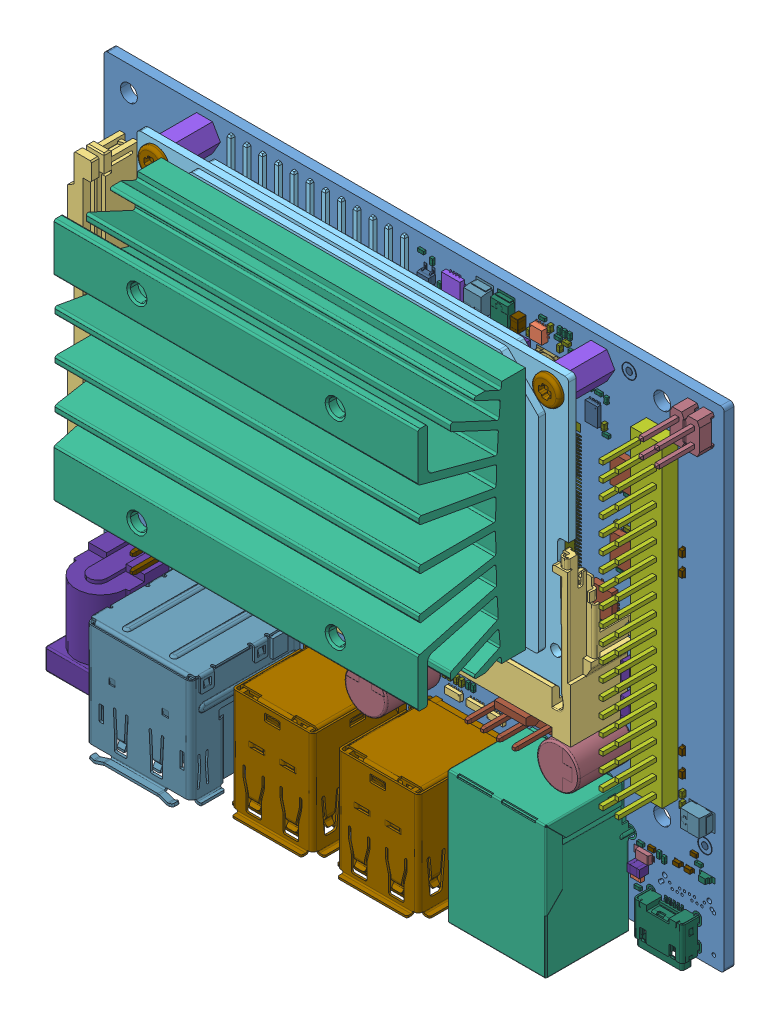
SolidWorks assembly Jetson_Nano_Dev_Kit_3D_b01, configuration Default. Lengths in mm. (continued)
Components (placement in the parent): (continued)
- Jetson_Nano_Dev_Kit_3D_b01(2)^Jetson_Nano_Dev_Kit_3D_b01-1: Jetson_Nano_Dev_Kit_3D_b01(2)^Jetson_Nano_Dev_Kit_3D_b01 [Default] at origin size (100 81.03 30.51) (virtual) (continued)
  - 642-13450_PORG_SYS_BOM^Jetson_Nano_Dev_Kit_3D_b01(2)_Jetson_Nano_Dev_Kit_3D_b01-1: 642-13450_PORG_SYS_BOM^Jetson_Nano_Dev_Kit_3D_b01(2)_Jetson_Nano_Dev_Kit_3D_b01 [Default] at origin size (100 81.03 23.18) (virtual) (continued)
    - 699-13449_PORG_DEV_KIT_PCB_ASSY^642-13450_PORG_SYS_BOM_Jetson_Nano_Dev_Kit_3D_b01(2)_Jetson_Nano_Dev_Kit_3D_b01-1: 699-13449_PORG_DEV_KIT_PCB_ASSY^642-13450_PORG_SYS_BOM_Jetson_Nano_Dev_Kit_3D_b01(2)_Jetson_Nano_Dev_Kit_3D_b01 [Default] at origin size (100 81.03 23.18) (virtual) (continued)
      - 600-13449_PORG_DEV_KIT_PCB_ASSY^699-13449_PORG_DEV_KIT_PCB_ASSY_642-13450_PORG_SYS_BOM_Jetson_Nano_Dev_Kit_3D_b01(2)_Jetson_Nano_Dev_Kit_3D_b01-1: 600-13449_PORG_DEV_KIT_PCB_ASSY^699-13449_PORG_DEV_KIT_PCB_ASSY_642-13450_PORG_SYS_BOM_Jetson_Nano_Dev_Kit_3D_b01(2)_Jetson_Nano_Dev_Kit_3D_b01 [Default] at origin size (100 81.03 23.18) (virtual) (continued)
        - 142-13449-1000-B01-SKU0000^600-13449_PORG_DEV_KIT_PCB_ASSY_699-13449_PORG_DEV_KIT_PCB_ASSY_642-13450_PORG_SYS_BOM_Jetson_Nano_Dev_Kit_3D_b01(2)_Jetson_Nano_Dev_Kit_3D_b01-1: 142-13449-1000-B01-SKU0000^600-13449_PORG_DEV_KIT_PCB_ASSY_699-13449_PORG_DEV_KIT_PCB_ASSY_642-13450_PORG_SYS_BOM_Jetson_Nano_Dev_Kit_3D_b01(2)_Jetson_Nano_Dev_Kit_3D_b01 [Default] at origin size (100 81.03 23.18) (virtual) (continued)
          - 0402_H060^142-13449-1000-B01-SKU0000_600-13449_PORG_DEV_KIT_PCB_ASSY_699-13449_PORG_DEV_KIT_PCB_ASSY_642-13450_PORG_SYS_BOM_Jetson_Nano_Dev_Kit_3D_b01(2)_Jetson_Nano_Dev_Kit_3D_b01-77: 0402_H060^142-13449-1000-B01-SKU0000_600-13449_PORG_DEV_KIT_PCB_ASSY_699-13449_PORG_DEV_KIT_PCB_ASSY_642-13450_PORG_SYS_BOM_Jetson_Nano_Dev_Kit_3D_b01(2)_Jetson_Nano_Dev_Kit_3D_b01 [Default] at (10.225 5.1 1.57) size (1 0.5 0.6) (virtual)
          - 0402_H060^142-13449-1000-B01-SKU0000_600-13449_PORG_DEV_KIT_PCB_ASSY_699-13449_PORG_DEV_KIT_PCB_ASSY_642-13450_PORG_SYS_BOM_Jetson_Nano_Dev_Kit_3D_b01(2)_Jetson_Nano_Dev_Kit_3D_b01-78: 0402_H060^142-13449-1000-B01-SKU0000_600-13449_PORG_DEV_KIT_PCB_ASSY_699-13449_PORG_DEV_KIT_PCB_ASSY_642-13450_PORG_SYS_BOM_Jetson_Nano_Dev_Kit_3D_b01(2)_Jetson_Nano_Dev_Kit_3D_b01 [Default] at (16.45 34.1 1.57) x (0 1 0) z (0 0 1) size (1 0.5 0.6) (virtual)
          - 0402_H040^142-13449-1000-B01-SKU0000_600-13449_PORG_DEV_KIT_PCB_ASSY_699-13449_PORG_DEV_KIT_PCB_ASSY_642-13450_PORG_SYS_BOM_Jetson_Nano_Dev_Kit_3D_b01(2)_Jetson_Nano_Dev_Kit_3D_b01-59: 0402_H040^142-13449-1000-B01-SKU0000_600-13449_PORG_DEV_KIT_PCB_ASSY_699-13449_PORG_DEV_KIT_PCB_ASSY_642-13450_PORG_SYS_BOM_Jetson_Nano_Dev_Kit_3D_b01(2)_Jetson_Nano_Dev_Kit_3D_b01 [Default] at (20.8 6.2 1.57) x (0 1 0) z (0 0 1) size (1 0.5 0.4) (virtual)
          - 0402_H040^142-13449-1000-B01-SKU0000_600-13449_PORG_DEV_KIT_PCB_ASSY_699-13449_PORG_DEV_KIT_PCB_ASSY_642-13450_PORG_SYS_BOM_Jetson_Nano_Dev_Kit_3D_b01(2)_Jetson_Nano_Dev_Kit_3D_b01-60: 0402_H040^142-13449-1000-B01-SKU0000_600-13449_PORG_DEV_KIT_PCB_ASSY_699-13449_PORG_DEV_KIT_PCB_ASSY_642-13450_PORG_SYS_BOM_Jetson_Nano_Dev_Kit_3D_b01(2)_Jetson_Nano_Dev_Kit_3D_b01 [Default] at (76 22.7 1.57) size (1 0.5 0.4) (virtual)
          - 0402_H040^142-13449-1000-B01-SKU0000_600-13449_PORG_DEV_KIT_PCB_ASSY_699-13449_PORG_DEV_KIT_PCB_ASSY_642-13450_PORG_SYS_BOM_Jetson_Nano_Dev_Kit_3D_b01(2)_Jetson_Nano_Dev_Kit_3D_b01-61: 0402_H040^142-13449-1000-B01-SKU0000_600-13449_PORG_DEV_KIT_PCB_ASSY_699-13449_PORG_DEV_KIT_PCB_ASSY_642-13450_PORG_SYS_BOM_Jetson_Nano_Dev_Kit_3D_b01(2)_Jetson_Nano_Dev_Kit_3D_b01 [Default] at (11.7 46.85 1.57) x (0 -1 0) z (0 0 1) size (1 0.5 0.4) (virtual)
          - 0402_H040^142-13449-1000-B01-SKU0000_600-13449_PORG_DEV_KIT_PCB_ASSY_699-13449_PORG_DEV_KIT_PCB_ASSY_642-13450_PORG_SYS_BOM_Jetson_Nano_Dev_Kit_3D_b01(2)_Jetson_Nano_Dev_Kit_3D_b01-62: 0402_H040^142-13449-1000-B01-SKU0000_600-13449_PORG_DEV_KIT_PCB_ASSY_699-13449_PORG_DEV_KIT_PCB_ASSY_642-13450_PORG_SYS_BOM_Jetson_Nano_Dev_Kit_3D_b01(2)_Jetson_Nano_Dev_Kit_3D_b01 [Default] at (12.75 46.85 1.57) x (0 -1 0) z (0 0 1) size (1 0.5 0.4) (virtual)
          - 0402_H040^142-13449-1000-B01-SKU0000_600-13449_PORG_DEV_KIT_PCB_ASSY_699-13449_PORG_DEV_KIT_PCB_ASSY_642-13450_PORG_SYS_BOM_Jetson_Nano_Dev_Kit_3D_b01(2)_Jetson_Nano_Dev_Kit_3D_b01-63: 0402_H040^142-13449-1000-B01-SKU0000_600-13449_PORG_DEV_KIT_PCB_ASSY_699-13449_PORG_DEV_KIT_PCB_ASSY_642-13450_PORG_SYS_BOM_Jetson_Nano_Dev_Kit_3D_b01(2)_Jetson_Nano_Dev_Kit_3D_b01 [Default] at (10 41.6 1.57) x (0 -1 0) z (0 0 1) size (1 0.5 0.4) (virtual)
          - 0402_H040^142-13449-1000-B01-SKU0000_600-13449_PORG_DEV_KIT_PCB_ASSY_699-13449_PORG_DEV_KIT_PCB_ASSY_642-13450_PORG_SYS_BOM_Jetson_Nano_Dev_Kit_3D_b01(2)_Jetson_Nano_Dev_Kit_3D_b01-64: 0402_H040^142-13449-1000-B01-SKU0000_600-13449_PORG_DEV_KIT_PCB_ASSY_699-13449_PORG_DEV_KIT_PCB_ASSY_642-13450_PORG_SYS_BOM_Jetson_Nano_Dev_Kit_3D_b01(2)_Jetson_Nano_Dev_Kit_3D_b01 [Default] at (13.15 4.2 1.57) x (0 -1 0) z (0 0 1) size (1 0.5 0.4) (virtual)
          - 0402_H040^142-13449-1000-B01-SKU0000_600-13449_PORG_DEV_KIT_PCB_ASSY_699-13449_PORG_DEV_KIT_PCB_ASSY_642-13450_PORG_SYS_BOM_Jetson_Nano_Dev_Kit_3D_b01(2)_Jetson_Nano_Dev_Kit_3D_b01-65: 0402_H040^142-13449-1000-B01-SKU0000_600-13449_PORG_DEV_KIT_PCB_ASSY_699-13449_PORG_DEV_KIT_PCB_ASSY_642-13450_PORG_SYS_BOM_Jetson_Nano_Dev_Kit_3D_b01(2)_Jetson_Nano_Dev_Kit_3D_b01 [Default] at (9.05 41.6 1.57) x (0 1 0) z (0 0 1) size (1 0.5 0.4) (virtual)
          - 0402_H040^142-13449-1000-B01-SKU0000_600-13449_PORG_DEV_KIT_PCB_ASSY_699-13449_PORG_DEV_KIT_PCB_ASSY_642-13450_PORG_SYS_BOM_Jetson_Nano_Dev_Kit_3D_b01(2)_Jetson_Nano_Dev_Kit_3D_b01-66: 0402_H040^142-13449-1000-B01-SKU0000_600-13449_PORG_DEV_KIT_PCB_ASSY_699-13449_PORG_DEV_KIT_PCB_ASSY_642-13450_PORG_SYS_BOM_Jetson_Nano_Dev_Kit_3D_b01(2)_Jetson_Nano_Dev_Kit_3D_b01 [Default] at (14.2 6.2 1.57) x (0 1 0) z (0 0 1) size (1 0.5 0.4) (virtual)
          - 0402_H040^142-13449-1000-B01-SKU0000_600-13449_PORG_DEV_KIT_PCB_ASSY_699-13449_PORG_DEV_KIT_PCB_ASSY_642-13450_PORG_SYS_BOM_Jetson_Nano_Dev_Kit_3D_b01(2)_Jetson_Nano_Dev_Kit_3D_b01-67: 0402_H040^142-13449-1000-B01-SKU0000_600-13449_PORG_DEV_KIT_PCB_ASSY_699-13449_PORG_DEV_KIT_PCB_ASSY_642-13450_PORG_SYS_BOM_Jetson_Nano_Dev_Kit_3D_b01(2)_Jetson_Nano_Dev_Kit_3D_b01 [Default] at (12.9 6.2 1.57) x (0 1 0) z (0 0 1) size (1 0.5 0.4) (virtual)
          - 0402_H040^142-13449-1000-B01-SKU0000_600-13449_PORG_DEV_KIT_PCB_ASSY_699-13449_PORG_DEV_KIT_PCB_ASSY_642-13450_PORG_SYS_BOM_Jetson_Nano_Dev_Kit_3D_b01(2)_Jetson_Nano_Dev_Kit_3D_b01-68: 0402_H040^142-13449-1000-B01-SKU0000_600-13449_PORG_DEV_KIT_PCB_ASSY_699-13449_PORG_DEV_KIT_PCB_ASSY_642-13450_PORG_SYS_BOM_Jetson_Nano_Dev_Kit_3D_b01(2)_Jetson_Nano_Dev_Kit_3D_b01 [Default] at (15.1 6.2 1.57) x (0 1 0) z (0 0 1) size (1 0.5 0.4) (virtual)
          - 0402_H040^142-13449-1000-B01-SKU0000_600-13449_PORG_DEV_KIT_PCB_ASSY_699-13449_PORG_DEV_KIT_PCB_ASSY_642-13450_PORG_SYS_BOM_Jetson_Nano_Dev_Kit_3D_b01(2)_Jetson_Nano_Dev_Kit_3D_b01-69: 0402_H040^142-13449-1000-B01-SKU0000_600-13449_PORG_DEV_KIT_PCB_ASSY_699-13449_PORG_DEV_KIT_PCB_ASSY_642-13450_PORG_SYS_BOM_Jetson_Nano_Dev_Kit_3D_b01(2)_Jetson_Nano_Dev_Kit_3D_b01 [Default] at (16.4 6.2 1.57) x (0 1 0) z (0 0 1) size (1 0.5 0.4) (virtual)
          - 0402_H040^142-13449-1000-B01-SKU0000_600-13449_PORG_DEV_KIT_PCB_ASSY_699-13449_PORG_DEV_KIT_PCB_ASSY_642-13450_PORG_SYS_BOM_Jetson_Nano_Dev_Kit_3D_b01(2)_Jetson_Nano_Dev_Kit_3D_b01-70: 0402_H040^142-13449-1000-B01-SKU0000_600-13449_PORG_DEV_KIT_PCB_ASSY_699-13449_PORG_DEV_KIT_PCB_ASSY_642-13450_PORG_SYS_BOM_Jetson_Nano_Dev_Kit_3D_b01(2)_Jetson_Nano_Dev_Kit_3D_b01 [Default] at (19.5 6.2 1.57) x (0 1 0) z (0 0 1) size (1 0.5 0.4) (virtual)
          - 0402_H040^142-13449-1000-B01-SKU0000_600-13449_PORG_DEV_KIT_PCB_ASSY_699-13449_PORG_DEV_KIT_PCB_ASSY_642-13450_PORG_SYS_BOM_Jetson_Nano_Dev_Kit_3D_b01(2)_Jetson_Nano_Dev_Kit_3D_b01-71: 0402_H040^142-13449-1000-B01-SKU0000_600-13449_PORG_DEV_KIT_PCB_ASSY_699-13449_PORG_DEV_KIT_PCB_ASSY_642-13450_PORG_SYS_BOM_Jetson_Nano_Dev_Kit_3D_b01(2)_Jetson_Nano_Dev_Kit_3D_b01 [Default] at (17.3 6.2 1.57) x (0 1 0) z (0 0 1) size (1 0.5 0.4) (virtual)
          - 0402_H040^142-13449-1000-B01-SKU0000_600-13449_PORG_DEV_KIT_PCB_ASSY_699-13449_PORG_DEV_KIT_PCB_ASSY_642-13450_PORG_SYS_BOM_Jetson_Nano_Dev_Kit_3D_b01(2)_Jetson_Nano_Dev_Kit_3D_b01-72: 0402_H040^142-13449-1000-B01-SKU0000_600-13449_PORG_DEV_KIT_PCB_ASSY_699-13449_PORG_DEV_KIT_PCB_ASSY_642-13450_PORG_SYS_BOM_Jetson_Nano_Dev_Kit_3D_b01(2)_Jetson_Nano_Dev_Kit_3D_b01 [Default] at (18.6 6.2 1.57) x (0 1 0) z (0 0 1) size (1 0.5 0.4) (virtual)
          - 0402_H040^142-13449-1000-B01-SKU0000_600-13449_PORG_DEV_KIT_PCB_ASSY_699-13449_PORG_DEV_KIT_PCB_ASSY_642-13450_PORG_SYS_BOM_Jetson_Nano_Dev_Kit_3D_b01(2)_Jetson_Nano_Dev_Kit_3D_b01-73: 0402_H040^142-13449-1000-B01-SKU0000_600-13449_PORG_DEV_KIT_PCB_ASSY_699-13449_PORG_DEV_KIT_PCB_ASSY_642-13450_PORG_SYS_BOM_Jetson_Nano_Dev_Kit_3D_b01(2)_Jetson_Nano_Dev_Kit_3D_b01 [Default] at (15.55 47.25 1.57) x (0 1 0) z (0 0 1) size (1 0.5 0.4) (virtual)
          - 0402_H040^142-13449-1000-B01-SKU0000_600-13449_PORG_DEV_KIT_PCB_ASSY_699-13449_PORG_DEV_KIT_PCB_ASSY_642-13450_PORG_SYS_BOM_Jetson_Nano_Dev_Kit_3D_b01(2)_Jetson_Nano_Dev_Kit_3D_b01-74: 0402_H040^142-13449-1000-B01-SKU0000_600-13449_PORG_DEV_KIT_PCB_ASSY_699-13449_PORG_DEV_KIT_PCB_ASSY_642-13450_PORG_SYS_BOM_Jetson_Nano_Dev_Kit_3D_b01(2)_Jetson_Nano_Dev_Kit_3D_b01 [Default] at (80.7 42.4 1.57) x (-1 0 0) z (0 0 1) size (1 0.5 0.4) (virtual)
          - 0402_H040^142-13449-1000-B01-SKU0000_600-13449_PORG_DEV_KIT_PCB_ASSY_699-13449_PORG_DEV_KIT_PCB_ASSY_642-13450_PORG_SYS_BOM_Jetson_Nano_Dev_Kit_3D_b01(2)_Jetson_Nano_Dev_Kit_3D_b01-75: 0402_H040^142-13449-1000-B01-SKU0000_600-13449_PORG_DEV_KIT_PCB_ASSY_699-13449_PORG_DEV_KIT_PCB_ASSY_642-13450_PORG_SYS_BOM_Jetson_Nano_Dev_Kit_3D_b01(2)_Jetson_Nano_Dev_Kit_3D_b01 [Default] at (77.5 22.7 1.57) x (-1 0 0) z (0 0 1) size (1 0.5 0.4) (virtual)
          - 0402_H040^142-13449-1000-B01-SKU0000_600-13449_PORG_DEV_KIT_PCB_ASSY_699-13449_PORG_DEV_KIT_PCB_ASSY_642-13450_PORG_SYS_BOM_Jetson_Nano_Dev_Kit_3D_b01(2)_Jetson_Nano_Dev_Kit_3D_b01-76: 0402_H040^142-13449-1000-B01-SKU0000_600-13449_PORG_DEV_KIT_PCB_ASSY_699-13449_PORG_DEV_KIT_PCB_ASSY_642-13450_PORG_SYS_BOM_Jetson_Nano_Dev_Kit_3D_b01(2)_Jetson_Nano_Dev_Kit_3D_b01 [Default] at (62.3 29.15 1.57) size (1 0.5 0.4) (virtual)
          - 0402_H040^142-13449-1000-B01-SKU0000_600-13449_PORG_DEV_KIT_PCB_ASSY_699-13449_PORG_DEV_KIT_PCB_ASSY_642-13450_PORG_SYS_BOM_Jetson_Nano_Dev_Kit_3D_b01(2)_Jetson_Nano_Dev_Kit_3D_b01-77: 0402_H040^142-13449-1000-B01-SKU0000_600-13449_PORG_DEV_KIT_PCB_ASSY_699-13449_PORG_DEV_KIT_PCB_ASSY_642-13450_PORG_SYS_BOM_Jetson_Nano_Dev_Kit_3D_b01(2)_Jetson_Nano_Dev_Kit_3D_b01 [Default] at (62.65 44.45 1.57) x (0 -1 0) z (0 0 1) size (1 0.5 0.4) (virtual)
          - 0402_H040^142-13449-1000-B01-SKU0000_600-13449_PORG_DEV_KIT_PCB_ASSY_699-13449_PORG_DEV_KIT_PCB_ASSY_642-13450_PORG_SYS_BOM_Jetson_Nano_Dev_Kit_3D_b01(2)_Jetson_Nano_Dev_Kit_3D_b01-78: 0402_H040^142-13449-1000-B01-SKU0000_600-13449_PORG_DEV_KIT_PCB_ASSY_699-13449_PORG_DEV_KIT_PCB_ASSY_642-13450_PORG_SYS_BOM_Jetson_Nano_Dev_Kit_3D_b01(2)_Jetson_Nano_Dev_Kit_3D_b01 [Default] at (62.85 27.15 1.57) size (1 0.5 0.4) (virtual)
          - 0402_H040^142-13449-1000-B01-SKU0000_600-13449_PORG_DEV_KIT_PCB_ASSY_699-13449_PORG_DEV_KIT_PCB_ASSY_642-13450_PORG_SYS_BOM_Jetson_Nano_Dev_Kit_3D_b01(2)_Jetson_Nano_Dev_Kit_3D_b01-79: 0402_H040^142-13449-1000-B01-SKU0000_600-13449_PORG_DEV_KIT_PCB_ASSY_699-13449_PORG_DEV_KIT_PCB_ASSY_642-13450_PORG_SYS_BOM_Jetson_Nano_Dev_Kit_3D_b01(2)_Jetson_Nano_Dev_Kit_3D_b01 [Default] at (32.85 5.81 1.57) x (0 -1 0) z (0 0 1) size (1 0.5 0.4) (virtual)
          - 0402_H040^142-13449-1000-B01-SKU0000_600-13449_PORG_DEV_KIT_PCB_ASSY_699-13449_PORG_DEV_KIT_PCB_ASSY_642-13450_PORG_SYS_BOM_Jetson_Nano_Dev_Kit_3D_b01(2)_Jetson_Nano_Dev_Kit_3D_b01-80: 0402_H040^142-13449-1000-B01-SKU0000_600-13449_PORG_DEV_KIT_PCB_ASSY_699-13449_PORG_DEV_KIT_PCB_ASSY_642-13450_PORG_SYS_BOM_Jetson_Nano_Dev_Kit_3D_b01(2)_Jetson_Nano_Dev_Kit_3D_b01 [Default] at (32.05 5.81 1.57) x (0 -1 0) z (0 0 1) size (1 0.5 0.4) (virtual)
          - 0402_H040^142-13449-1000-B01-SKU0000_600-13449_PORG_DEV_KIT_PCB_ASSY_699-13449_PORG_DEV_KIT_PCB_ASSY_642-13450_PORG_SYS_BOM_Jetson_Nano_Dev_Kit_3D_b01(2)_Jetson_Nano_Dev_Kit_3D_b01-81: 0402_H040^142-13449-1000-B01-SKU0000_600-13449_PORG_DEV_KIT_PCB_ASSY_699-13449_PORG_DEV_KIT_PCB_ASSY_642-13450_PORG_SYS_BOM_Jetson_Nano_Dev_Kit_3D_b01(2)_Jetson_Nano_Dev_Kit_3D_b01 [Default] at (27.25 5.81 1.57) x (0 -1 0) z (0 0 1) size (1 0.5 0.4) (virtual)
          - 0402_H040^142-13449-1000-B01-SKU0000_600-13449_PORG_DEV_KIT_PCB_ASSY_699-13449_PORG_DEV_KIT_PCB_ASSY_642-13450_PORG_SYS_BOM_Jetson_Nano_Dev_Kit_3D_b01(2)_Jetson_Nano_Dev_Kit_3D_b01-82: 0402_H040^142-13449-1000-B01-SKU0000_600-13449_PORG_DEV_KIT_PCB_ASSY_699-13449_PORG_DEV_KIT_PCB_ASSY_642-13450_PORG_SYS_BOM_Jetson_Nano_Dev_Kit_3D_b01(2)_Jetson_Nano_Dev_Kit_3D_b01 [Default] at (28.05 5.81 1.57) x (0 -1 0) z (0 0 1) size (1 0.5 0.4) (virtual)
          - 0402_H040^142-13449-1000-B01-SKU0000_600-13449_PORG_DEV_KIT_PCB_ASSY_699-13449_PORG_DEV_KIT_PCB_ASSY_642-13450_PORG_SYS_BOM_Jetson_Nano_Dev_Kit_3D_b01(2)_Jetson_Nano_Dev_Kit_3D_b01-83: 0402_H040^142-13449-1000-B01-SKU0000_600-13449_PORG_DEV_KIT_PCB_ASSY_699-13449_PORG_DEV_KIT_PCB_ASSY_642-13450_PORG_SYS_BOM_Jetson_Nano_Dev_Kit_3D_b01(2)_Jetson_Nano_Dev_Kit_3D_b01 [Default] at (31.25 5.81 1.57) x (0 -1 0) z (0 0 1) size (1 0.5 0.4) (virtual)
          - 0402_H040^142-13449-1000-B01-SKU0000_600-13449_PORG_DEV_KIT_PCB_ASSY_699-13449_PORG_DEV_KIT_PCB_ASSY_642-13450_PORG_SYS_BOM_Jetson_Nano_Dev_Kit_3D_b01(2)_Jetson_Nano_Dev_Kit_3D_b01-84: 0402_H040^142-13449-1000-B01-SKU0000_600-13449_PORG_DEV_KIT_PCB_ASSY_699-13449_PORG_DEV_KIT_PCB_ASSY_642-13450_PORG_SYS_BOM_Jetson_Nano_Dev_Kit_3D_b01(2)_Jetson_Nano_Dev_Kit_3D_b01 [Default] at (30.45 5.81 1.57) x (0 -1 0) z (0 0 1) size (1 0.5 0.4) (virtual)
          - 0402_H040^142-13449-1000-B01-SKU0000_600-13449_PORG_DEV_KIT_PCB_ASSY_699-13449_PORG_DEV_KIT_PCB_ASSY_642-13450_PORG_SYS_BOM_Jetson_Nano_Dev_Kit_3D_b01(2)_Jetson_Nano_Dev_Kit_3D_b01-85: 0402_H040^142-13449-1000-B01-SKU0000_600-13449_PORG_DEV_KIT_PCB_ASSY_699-13449_PORG_DEV_KIT_PCB_ASSY_642-13450_PORG_SYS_BOM_Jetson_Nano_Dev_Kit_3D_b01(2)_Jetson_Nano_Dev_Kit_3D_b01 [Default] at (28.85 5.81 1.57) x (0 -1 0) z (0 0 1) size (1 0.5 0.4) (virtual)
          - 0402_H040^142-13449-1000-B01-SKU0000_600-13449_PORG_DEV_KIT_PCB_ASSY_699-13449_PORG_DEV_KIT_PCB_ASSY_642-13450_PORG_SYS_BOM_Jetson_Nano_Dev_Kit_3D_b01(2)_Jetson_Nano_Dev_Kit_3D_b01-86: 0402_H040^142-13449-1000-B01-SKU0000_600-13449_PORG_DEV_KIT_PCB_ASSY_699-13449_PORG_DEV_KIT_PCB_ASSY_642-13450_PORG_SYS_BOM_Jetson_Nano_Dev_Kit_3D_b01(2)_Jetson_Nano_Dev_Kit_3D_b01 [Default] at (29.65 5.81 1.57) x (0 -1 0) z (0 0 1) size (1 0.5 0.4) (virtual)
          - 0402_H040^142-13449-1000-B01-SKU0000_600-13449_PORG_DEV_KIT_PCB_ASSY_699-13449_PORG_DEV_KIT_PCB_ASSY_642-13450_PORG_SYS_BOM_Jetson_Nano_Dev_Kit_3D_b01(2)_Jetson_Nano_Dev_Kit_3D_b01-87: 0402_H040^142-13449-1000-B01-SKU0000_600-13449_PORG_DEV_KIT_PCB_ASSY_699-13449_PORG_DEV_KIT_PCB_ASSY_642-13450_PORG_SYS_BOM_Jetson_Nano_Dev_Kit_3D_b01(2)_Jetson_Nano_Dev_Kit_3D_b01 [Default] at (44.4 46.4 1.57) x (0 1 0) z (0 0 1) size (1 0.5 0.4) (virtual)
          - 0402_H040^142-13449-1000-B01-SKU0000_600-13449_PORG_DEV_KIT_PCB_ASSY_699-13449_PORG_DEV_KIT_PCB_ASSY_642-13450_PORG_SYS_BOM_Jetson_Nano_Dev_Kit_3D_b01(2)_Jetson_Nano_Dev_Kit_3D_b01-88: 0402_H040^142-13449-1000-B01-SKU0000_600-13449_PORG_DEV_KIT_PCB_ASSY_699-13449_PORG_DEV_KIT_PCB_ASSY_642-13450_PORG_SYS_BOM_Jetson_Nano_Dev_Kit_3D_b01(2)_Jetson_Nano_Dev_Kit_3D_b01 [Default] at (25.85 4.9 1.57) x (0 -1 0) z (0 0 1) size (1 0.5 0.4) (virtual)
          - 0402_H040^142-13449-1000-B01-SKU0000_600-13449_PORG_DEV_KIT_PCB_ASSY_699-13449_PORG_DEV_KIT_PCB_ASSY_642-13450_PORG_SYS_BOM_Jetson_Nano_Dev_Kit_3D_b01(2)_Jetson_Nano_Dev_Kit_3D_b01-89: 0402_H040^142-13449-1000-B01-SKU0000_600-13449_PORG_DEV_KIT_PCB_ASSY_699-13449_PORG_DEV_KIT_PCB_ASSY_642-13450_PORG_SYS_BOM_Jetson_Nano_Dev_Kit_3D_b01(2)_Jetson_Nano_Dev_Kit_3D_b01 [Default] at (43.4 46.4 1.57) x (0 1 0) z (0 0 1) size (1 0.5 0.4) (virtual)
          - 0402_H040^142-13449-1000-B01-SKU0000_600-13449_PORG_DEV_KIT_PCB_ASSY_699-13449_PORG_DEV_KIT_PCB_ASSY_642-13450_PORG_SYS_BOM_Jetson_Nano_Dev_Kit_3D_b01(2)_Jetson_Nano_Dev_Kit_3D_b01-90: 0402_H040^142-13449-1000-B01-SKU0000_600-13449_PORG_DEV_KIT_PCB_ASSY_699-13449_PORG_DEV_KIT_PCB_ASSY_642-13450_PORG_SYS_BOM_Jetson_Nano_Dev_Kit_3D_b01(2)_Jetson_Nano_Dev_Kit_3D_b01 [Default] at (82.8 -5.3 1.57) x (-1 0 0) z (0 0 1) size (1 0.5 0.4) (virtual)
          - 0402_H040^142-13449-1000-B01-SKU0000_600-13449_PORG_DEV_KIT_PCB_ASSY_699-13449_PORG_DEV_KIT_PCB_ASSY_642-13450_PORG_SYS_BOM_Jetson_Nano_Dev_Kit_3D_b01(2)_Jetson_Nano_Dev_Kit_3D_b01-91: 0402_H040^142-13449-1000-B01-SKU0000_600-13449_PORG_DEV_KIT_PCB_ASSY_699-13449_PORG_DEV_KIT_PCB_ASSY_642-13450_PORG_SYS_BOM_Jetson_Nano_Dev_Kit_3D_b01(2)_Jetson_Nano_Dev_Kit_3D_b01 [Default] at (82.4 -11.6 1.57) x (-1 0 0) z (0 0 1) size (1 0.5 0.4) (virtual)
          - 0402_H040^142-13449-1000-B01-SKU0000_600-13449_PORG_DEV_KIT_PCB_ASSY_699-13449_PORG_DEV_KIT_PCB_ASSY_642-13450_PORG_SYS_BOM_Jetson_Nano_Dev_Kit_3D_b01(2)_Jetson_Nano_Dev_Kit_3D_b01-92: 0402_H040^142-13449-1000-B01-SKU0000_600-13449_PORG_DEV_KIT_PCB_ASSY_699-13449_PORG_DEV_KIT_PCB_ASSY_642-13450_PORG_SYS_BOM_Jetson_Nano_Dev_Kit_3D_b01(2)_Jetson_Nano_Dev_Kit_3D_b01 [Default] at (38.45 47.85 1.57) x (-1 0 0) z (0 0 1) size (1 0.5 0.4) (virtual)
          - 0402_H040^142-13449-1000-B01-SKU0000_600-13449_PORG_DEV_KIT_PCB_ASSY_699-13449_PORG_DEV_KIT_PCB_ASSY_642-13450_PORG_SYS_BOM_Jetson_Nano_Dev_Kit_3D_b01(2)_Jetson_Nano_Dev_Kit_3D_b01-93: 0402_H040^142-13449-1000-B01-SKU0000_600-13449_PORG_DEV_KIT_PCB_ASSY_699-13449_PORG_DEV_KIT_PCB_ASSY_642-13450_PORG_SYS_BOM_Jetson_Nano_Dev_Kit_3D_b01(2)_Jetson_Nano_Dev_Kit_3D_b01 [Default] at (33.8 43.1 1.57) size (1 0.5 0.4) (virtual)
          - 0402_H040^142-13449-1000-B01-SKU0000_600-13449_PORG_DEV_KIT_PCB_ASSY_699-13449_PORG_DEV_KIT_PCB_ASSY_642-13450_PORG_SYS_BOM_Jetson_Nano_Dev_Kit_3D_b01(2)_Jetson_Nano_Dev_Kit_3D_b01-94: 0402_H040^142-13449-1000-B01-SKU0000_600-13449_PORG_DEV_KIT_PCB_ASSY_699-13449_PORG_DEV_KIT_PCB_ASSY_642-13450_PORG_SYS_BOM_Jetson_Nano_Dev_Kit_3D_b01(2)_Jetson_Nano_Dev_Kit_3D_b01 [Default] at (24.65 4.9 1.57) x (0 1 0) z (0 0 1) size (1 0.5 0.4) (virtual)
          - 0402_H040^142-13449-1000-B01-SKU0000_600-13449_PORG_DEV_KIT_PCB_ASSY_699-13449_PORG_DEV_KIT_PCB_ASSY_642-13450_PORG_SYS_BOM_Jetson_Nano_Dev_Kit_3D_b01(2)_Jetson_Nano_Dev_Kit_3D_b01-95: 0402_H040^142-13449-1000-B01-SKU0000_600-13449_PORG_DEV_KIT_PCB_ASSY_699-13449_PORG_DEV_KIT_PCB_ASSY_642-13450_PORG_SYS_BOM_Jetson_Nano_Dev_Kit_3D_b01(2)_Jetson_Nano_Dev_Kit_3D_b01 [Default] at (33.8 7.4 1.57) x (0 1 0) z (0 0 1) size (1 0.5 0.4) (virtual)
          - 0402_H040^142-13449-1000-B01-SKU0000_600-13449_PORG_DEV_KIT_PCB_ASSY_699-13449_PORG_DEV_KIT_PCB_ASSY_642-13450_PORG_SYS_BOM_Jetson_Nano_Dev_Kit_3D_b01(2)_Jetson_Nano_Dev_Kit_3D_b01-96: 0402_H040^142-13449-1000-B01-SKU0000_600-13449_PORG_DEV_KIT_PCB_ASSY_699-13449_PORG_DEV_KIT_PCB_ASSY_642-13450_PORG_SYS_BOM_Jetson_Nano_Dev_Kit_3D_b01(2)_Jetson_Nano_Dev_Kit_3D_b01 [Default] at (79.2 42.4 1.57) size (1 0.5 0.4) (virtual)
          - 0402_H040^142-13449-1000-B01-SKU0000_600-13449_PORG_DEV_KIT_PCB_ASSY_699-13449_PORG_DEV_KIT_PCB_ASSY_642-13450_PORG_SYS_BOM_Jetson_Nano_Dev_Kit_3D_b01(2)_Jetson_Nano_Dev_Kit_3D_b01-97: 0402_H040^142-13449-1000-B01-SKU0000_600-13449_PORG_DEV_KIT_PCB_ASSY_699-13449_PORG_DEV_KIT_PCB_ASSY_642-13450_PORG_SYS_BOM_Jetson_Nano_Dev_Kit_3D_b01(2)_Jetson_Nano_Dev_Kit_3D_b01 [Default] at (16.75 45.2 1.57) size (1 0.5 0.4) (virtual)
          - 0402_H040^142-13449-1000-B01-SKU0000_600-13449_PORG_DEV_KIT_PCB_ASSY_699-13449_PORG_DEV_KIT_PCB_ASSY_642-13450_PORG_SYS_BOM_Jetson_Nano_Dev_Kit_3D_b01(2)_Jetson_Nano_Dev_Kit_3D_b01-98: 0402_H040^142-13449-1000-B01-SKU0000_600-13449_PORG_DEV_KIT_PCB_ASSY_699-13449_PORG_DEV_KIT_PCB_ASSY_642-13450_PORG_SYS_BOM_Jetson_Nano_Dev_Kit_3D_b01(2)_Jetson_Nano_Dev_Kit_3D_b01 [Default] at (9.65 9.7 1.57) x (0 -1 0) z (0 0 1) size (1 0.5 0.4) (virtual)
          - 0402_H040^142-13449-1000-B01-SKU0000_600-13449_PORG_DEV_KIT_PCB_ASSY_699-13449_PORG_DEV_KIT_PCB_ASSY_642-13450_PORG_SYS_BOM_Jetson_Nano_Dev_Kit_3D_b01(2)_Jetson_Nano_Dev_Kit_3D_b01-99: 0402_H040^142-13449-1000-B01-SKU0000_600-13449_PORG_DEV_KIT_PCB_ASSY_699-13449_PORG_DEV_KIT_PCB_ASSY_642-13450_PORG_SYS_BOM_Jetson_Nano_Dev_Kit_3D_b01(2)_Jetson_Nano_Dev_Kit_3D_b01 [Default] at (23.7 28.55 1.57) x (0 1 0) z (0 0 1) size (1 0.5 0.4) (virtual)
          - 0402_H040^142-13449-1000-B01-SKU0000_600-13449_PORG_DEV_KIT_PCB_ASSY_699-13449_PORG_DEV_KIT_PCB_ASSY_642-13450_PORG_SYS_BOM_Jetson_Nano_Dev_Kit_3D_b01(2)_Jetson_Nano_Dev_Kit_3D_b01-100: 0402_H040^142-13449-1000-B01-SKU0000_600-13449_PORG_DEV_KIT_PCB_ASSY_699-13449_PORG_DEV_KIT_PCB_ASSY_642-13450_PORG_SYS_BOM_Jetson_Nano_Dev_Kit_3D_b01(2)_Jetson_Nano_Dev_Kit_3D_b01 [Default] at (10.625 6.35 1.57) x (0 -1 0) z (0 0 1) size (1 0.5 0.4) (virtual)
          - 0402_H040^142-13449-1000-B01-SKU0000_600-13449_PORG_DEV_KIT_PCB_ASSY_699-13449_PORG_DEV_KIT_PCB_ASSY_642-13450_PORG_SYS_BOM_Jetson_Nano_Dev_Kit_3D_b01(2)_Jetson_Nano_Dev_Kit_3D_b01-101: 0402_H040^142-13449-1000-B01-SKU0000_600-13449_PORG_DEV_KIT_PCB_ASSY_699-13449_PORG_DEV_KIT_PCB_ASSY_642-13450_PORG_SYS_BOM_Jetson_Nano_Dev_Kit_3D_b01(2)_Jetson_Nano_Dev_Kit_3D_b01 [Default] at (9.825 6.35 1.57) x (0 1 0) z (0 0 1) size (1 0.5 0.4) (virtual)
          - 0402_H040^142-13449-1000-B01-SKU0000_600-13449_PORG_DEV_KIT_PCB_ASSY_699-13449_PORG_DEV_KIT_PCB_ASSY_642-13450_PORG_SYS_BOM_Jetson_Nano_Dev_Kit_3D_b01(2)_Jetson_Nano_Dev_Kit_3D_b01-102: 0402_H040^142-13449-1000-B01-SKU0000_600-13449_PORG_DEV_KIT_PCB_ASSY_699-13449_PORG_DEV_KIT_PCB_ASSY_642-13450_PORG_SYS_BOM_Jetson_Nano_Dev_Kit_3D_b01(2)_Jetson_Nano_Dev_Kit_3D_b01 [Default] at (38.5 44.85 1.57) x (-1 0 0) z (0 0 1) size (1 0.5 0.4) (virtual)
          - 0402_H040^142-13449-1000-B01-SKU0000_600-13449_PORG_DEV_KIT_PCB_ASSY_699-13449_PORG_DEV_KIT_PCB_ASSY_642-13450_PORG_SYS_BOM_Jetson_Nano_Dev_Kit_3D_b01(2)_Jetson_Nano_Dev_Kit_3D_b01-103: 0402_H040^142-13449-1000-B01-SKU0000_600-13449_PORG_DEV_KIT_PCB_ASSY_699-13449_PORG_DEV_KIT_PCB_ASSY_642-13450_PORG_SYS_BOM_Jetson_Nano_Dev_Kit_3D_b01(2)_Jetson_Nano_Dev_Kit_3D_b01 [Default] at (11.9 33.55 1.57) size (1 0.5 0.4) (virtual)
          - 0402_H040^142-13449-1000-B01-SKU0000_600-13449_PORG_DEV_KIT_PCB_ASSY_699-13449_PORG_DEV_KIT_PCB_ASSY_642-13450_PORG_SYS_BOM_Jetson_Nano_Dev_Kit_3D_b01(2)_Jetson_Nano_Dev_Kit_3D_b01-104: 0402_H040^142-13449-1000-B01-SKU0000_600-13449_PORG_DEV_KIT_PCB_ASSY_699-13449_PORG_DEV_KIT_PCB_ASSY_642-13450_PORG_SYS_BOM_Jetson_Nano_Dev_Kit_3D_b01(2)_Jetson_Nano_Dev_Kit_3D_b01 [Default] at (11.65 44.85 1.57) x (0 1 0) z (0 0 1) size (1 0.5 0.4) (virtual)
          - 0402_H040^142-13449-1000-B01-SKU0000_600-13449_PORG_DEV_KIT_PCB_ASSY_699-13449_PORG_DEV_KIT_PCB_ASSY_642-13450_PORG_SYS_BOM_Jetson_Nano_Dev_Kit_3D_b01(2)_Jetson_Nano_Dev_Kit_3D_b01-105: 0402_H040^142-13449-1000-B01-SKU0000_600-13449_PORG_DEV_KIT_PCB_ASSY_699-13449_PORG_DEV_KIT_PCB_ASSY_642-13450_PORG_SYS_BOM_Jetson_Nano_Dev_Kit_3D_b01(2)_Jetson_Nano_Dev_Kit_3D_b01 [Default] at (77.3 49 1.57) size (1 0.5 0.4) (virtual)
          - 0402_H040^142-13449-1000-B01-SKU0000_600-13449_PORG_DEV_KIT_PCB_ASSY_699-13449_PORG_DEV_KIT_PCB_ASSY_642-13450_PORG_SYS_BOM_Jetson_Nano_Dev_Kit_3D_b01(2)_Jetson_Nano_Dev_Kit_3D_b01-106: 0402_H040^142-13449-1000-B01-SKU0000_600-13449_PORG_DEV_KIT_PCB_ASSY_699-13449_PORG_DEV_KIT_PCB_ASSY_642-13450_PORG_SYS_BOM_Jetson_Nano_Dev_Kit_3D_b01(2)_Jetson_Nano_Dev_Kit_3D_b01 [Default] at (74.6 54.3 1.57) size (1 0.5 0.4) (virtual)
          - 0402_H040^142-13449-1000-B01-SKU0000_600-13449_PORG_DEV_KIT_PCB_ASSY_699-13449_PORG_DEV_KIT_PCB_ASSY_642-13450_PORG_SYS_BOM_Jetson_Nano_Dev_Kit_3D_b01(2)_Jetson_Nano_Dev_Kit_3D_b01-107: 0402_H040^142-13449-1000-B01-SKU0000_600-13449_PORG_DEV_KIT_PCB_ASSY_699-13449_PORG_DEV_KIT_PCB_ASSY_642-13450_PORG_SYS_BOM_Jetson_Nano_Dev_Kit_3D_b01(2)_Jetson_Nano_Dev_Kit_3D_b01 [Default] at (13.1 33.15 1.57) x (0 -1 0) z (0 0 1) size (1 0.5 0.4) (virtual)
          - 0402_H040^142-13449-1000-B01-SKU0000_600-13449_PORG_DEV_KIT_PCB_ASSY_699-13449_PORG_DEV_KIT_PCB_ASSY_642-13450_PORG_SYS_BOM_Jetson_Nano_Dev_Kit_3D_b01(2)_Jetson_Nano_Dev_Kit_3D_b01-108: 0402_H040^142-13449-1000-B01-SKU0000_600-13449_PORG_DEV_KIT_PCB_ASSY_699-13449_PORG_DEV_KIT_PCB_ASSY_642-13450_PORG_SYS_BOM_Jetson_Nano_Dev_Kit_3D_b01(2)_Jetson_Nano_Dev_Kit_3D_b01 [Default] at (17.75 28.55 1.57) x (0 1 0) z (0 0 1) size (1 0.5 0.4) (virtual)
          - 0402_H040^142-13449-1000-B01-SKU0000_600-13449_PORG_DEV_KIT_PCB_ASSY_699-13449_PORG_DEV_KIT_PCB_ASSY_642-13450_PORG_SYS_BOM_Jetson_Nano_Dev_Kit_3D_b01(2)_Jetson_Nano_Dev_Kit_3D_b01-109: 0402_H040^142-13449-1000-B01-SKU0000_600-13449_PORG_DEV_KIT_PCB_ASSY_699-13449_PORG_DEV_KIT_PCB_ASSY_642-13450_PORG_SYS_BOM_Jetson_Nano_Dev_Kit_3D_b01(2)_Jetson_Nano_Dev_Kit_3D_b01 [Default] at (24.85 48.25 1.57) x (0 1 0) z (0 0 1) size (1 0.5 0.4) (virtual)
          - 0402_H040^142-13449-1000-B01-SKU0000_600-13449_PORG_DEV_KIT_PCB_ASSY_699-13449_PORG_DEV_KIT_PCB_ASSY_642-13450_PORG_SYS_BOM_Jetson_Nano_Dev_Kit_3D_b01(2)_Jetson_Nano_Dev_Kit_3D_b01-110: 0402_H040^142-13449-1000-B01-SKU0000_600-13449_PORG_DEV_KIT_PCB_ASSY_699-13449_PORG_DEV_KIT_PCB_ASSY_642-13450_PORG_SYS_BOM_Jetson_Nano_Dev_Kit_3D_b01(2)_Jetson_Nano_Dev_Kit_3D_b01 [Default] at (77.3 53.9 1.57) x (0 -1 0) z (0 0 1) size (1 0.5 0.4) (virtual)
          - 0402_H040^142-13449-1000-B01-SKU0000_600-13449_PORG_DEV_KIT_PCB_ASSY_699-13449_PORG_DEV_KIT_PCB_ASSY_642-13450_PORG_SYS_BOM_Jetson_Nano_Dev_Kit_3D_b01(2)_Jetson_Nano_Dev_Kit_3D_b01-111: 0402_H040^142-13449-1000-B01-SKU0000_600-13449_PORG_DEV_KIT_PCB_ASSY_699-13449_PORG_DEV_KIT_PCB_ASSY_642-13450_PORG_SYS_BOM_Jetson_Nano_Dev_Kit_3D_b01(2)_Jetson_Nano_Dev_Kit_3D_b01 [Default] at (76.1 54.3 1.57) x (-1 0 0) z (0 0 1) size (1 0.5 0.4) (virtual)
          - 0402_H040^142-13449-1000-B01-SKU0000_600-13449_PORG_DEV_KIT_PCB_ASSY_699-13449_PORG_DEV_KIT_PCB_ASSY_642-13450_PORG_SYS_BOM_Jetson_Nano_Dev_Kit_3D_b01(2)_Jetson_Nano_Dev_Kit_3D_b01-112: 0402_H040^142-13449-1000-B01-SKU0000_600-13449_PORG_DEV_KIT_PCB_ASSY_699-13449_PORG_DEV_KIT_PCB_ASSY_642-13450_PORG_SYS_BOM_Jetson_Nano_Dev_Kit_3D_b01(2)_Jetson_Nano_Dev_Kit_3D_b01 [Default] at (86.6 -5.6 1.57) x (0 1 0) z (0 0 1) size (1 0.5 0.4) (virtual)
          - 0402_H040^142-13449-1000-B01-SKU0000_600-13449_PORG_DEV_KIT_PCB_ASSY_699-13449_PORG_DEV_KIT_PCB_ASSY_642-13450_PORG_SYS_BOM_Jetson_Nano_Dev_Kit_3D_b01(2)_Jetson_Nano_Dev_Kit_3D_b01-113: 0402_H040^142-13449-1000-B01-SKU0000_600-13449_PORG_DEV_KIT_PCB_ASSY_699-13449_PORG_DEV_KIT_PCB_ASSY_642-13450_PORG_SYS_BOM_Jetson_Nano_Dev_Kit_3D_b01(2)_Jetson_Nano_Dev_Kit_3D_b01 [Default] at (85.8 -5.3 1.57) x (0 1 0) z (0 0 1) size (1 0.5 0.4) (virtual)
          - 0402_H040^142-13449-1000-B01-SKU0000_600-13449_PORG_DEV_KIT_PCB_ASSY_699-13449_PORG_DEV_KIT_PCB_ASSY_642-13450_PORG_SYS_BOM_Jetson_Nano_Dev_Kit_3D_b01(2)_Jetson_Nano_Dev_Kit_3D_b01-114: 0402_H040^142-13449-1000-B01-SKU0000_600-13449_PORG_DEV_KIT_PCB_ASSY_699-13449_PORG_DEV_KIT_PCB_ASSY_642-13450_PORG_SYS_BOM_Jetson_Nano_Dev_Kit_3D_b01(2)_Jetson_Nano_Dev_Kit_3D_b01 [Default] at (40.4 48.5 1.57) size (1 0.5 0.4) (virtual)
          - 0402_H040^142-13449-1000-B01-SKU0000_600-13449_PORG_DEV_KIT_PCB_ASSY_699-13449_PORG_DEV_KIT_PCB_ASSY_642-13450_PORG_SYS_BOM_Jetson_Nano_Dev_Kit_3D_b01(2)_Jetson_Nano_Dev_Kit_3D_b01-115: 0402_H040^142-13449-1000-B01-SKU0000_600-13449_PORG_DEV_KIT_PCB_ASSY_699-13449_PORG_DEV_KIT_PCB_ASSY_642-13450_PORG_SYS_BOM_Jetson_Nano_Dev_Kit_3D_b01(2)_Jetson_Nano_Dev_Kit_3D_b01 [Default] at (13.95 4.2 1.57) x (0 -1 0) z (0 0 1) size (1 0.5 0.4) (virtual)
          - 0402_H040^142-13449-1000-B01-SKU0000_600-13449_PORG_DEV_KIT_PCB_ASSY_699-13449_PORG_DEV_KIT_PCB_ASSY_642-13450_PORG_SYS_BOM_Jetson_Nano_Dev_Kit_3D_b01(2)_Jetson_Nano_Dev_Kit_3D_b01-116: 0402_H040^142-13449-1000-B01-SKU0000_600-13449_PORG_DEV_KIT_PCB_ASSY_699-13449_PORG_DEV_KIT_PCB_ASSY_642-13450_PORG_SYS_BOM_Jetson_Nano_Dev_Kit_3D_b01(2)_Jetson_Nano_Dev_Kit_3D_b01 [Default] at (15.35 4.2 1.57) x (0 -1 0) z (0 0 1) size (1 0.5 0.4) (virtual)
          - 0402_H040^142-13449-1000-B01-SKU0000_600-13449_PORG_DEV_KIT_PCB_ASSY_699-13449_PORG_DEV_KIT_PCB_ASSY_642-13450_PORG_SYS_BOM_Jetson_Nano_Dev_Kit_3D_b01(2)_Jetson_Nano_Dev_Kit_3D_b01-117: 0402_H040^142-13449-1000-B01-SKU0000_600-13449_PORG_DEV_KIT_PCB_ASSY_699-13449_PORG_DEV_KIT_PCB_ASSY_642-13450_PORG_SYS_BOM_Jetson_Nano_Dev_Kit_3D_b01(2)_Jetson_Nano_Dev_Kit_3D_b01 [Default] at (16.15 4.2 1.57) x (0 -1 0) z (0 0 1) size (1 0.5 0.4) (virtual)
          - 0402_H040^142-13449-1000-B01-SKU0000_600-13449_PORG_DEV_KIT_PCB_ASSY_699-13449_PORG_DEV_KIT_PCB_ASSY_642-13450_PORG_SYS_BOM_Jetson_Nano_Dev_Kit_3D_b01(2)_Jetson_Nano_Dev_Kit_3D_b01-118: 0402_H040^142-13449-1000-B01-SKU0000_600-13449_PORG_DEV_KIT_PCB_ASSY_699-13449_PORG_DEV_KIT_PCB_ASSY_642-13450_PORG_SYS_BOM_Jetson_Nano_Dev_Kit_3D_b01(2)_Jetson_Nano_Dev_Kit_3D_b01 [Default] at (20.55 4.2 1.57) x (0 -1 0) z (0 0 1) size (1 0.5 0.4) (virtual)
          - 0402_H040^142-13449-1000-B01-SKU0000_600-13449_PORG_DEV_KIT_PCB_ASSY_699-13449_PORG_DEV_KIT_PCB_ASSY_642-13450_PORG_SYS_BOM_Jetson_Nano_Dev_Kit_3D_b01(2)_Jetson_Nano_Dev_Kit_3D_b01-119: 0402_H040^142-13449-1000-B01-SKU0000_600-13449_PORG_DEV_KIT_PCB_ASSY_699-13449_PORG_DEV_KIT_PCB_ASSY_642-13450_PORG_SYS_BOM_Jetson_Nano_Dev_Kit_3D_b01(2)_Jetson_Nano_Dev_Kit_3D_b01 [Default] at (19.75 4.2 1.57) x (0 -1 0) z (0 0 1) size (1 0.5 0.4) (virtual)
          - 0402_H040^142-13449-1000-B01-SKU0000_600-13449_PORG_DEV_KIT_PCB_ASSY_699-13449_PORG_DEV_KIT_PCB_ASSY_642-13450_PORG_SYS_BOM_Jetson_Nano_Dev_Kit_3D_b01(2)_Jetson_Nano_Dev_Kit_3D_b01-120: 0402_H040^142-13449-1000-B01-SKU0000_600-13449_PORG_DEV_KIT_PCB_ASSY_699-13449_PORG_DEV_KIT_PCB_ASSY_642-13450_PORG_SYS_BOM_Jetson_Nano_Dev_Kit_3D_b01(2)_Jetson_Nano_Dev_Kit_3D_b01 [Default] at (17.6 4.2 1.57) x (0 -1 0) z (0 0 1) size (1 0.5 0.4) (virtual)
          - 0402_H040^142-13449-1000-B01-SKU0000_600-13449_PORG_DEV_KIT_PCB_ASSY_699-13449_PORG_DEV_KIT_PCB_ASSY_642-13450_PORG_SYS_BOM_Jetson_Nano_Dev_Kit_3D_b01(2)_Jetson_Nano_Dev_Kit_3D_b01-121: 0402_H040^142-13449-1000-B01-SKU0000_600-13449_PORG_DEV_KIT_PCB_ASSY_699-13449_PORG_DEV_KIT_PCB_ASSY_642-13450_PORG_SYS_BOM_Jetson_Nano_Dev_Kit_3D_b01(2)_Jetson_Nano_Dev_Kit_3D_b01 [Default] at (18.4 4.2 1.57) x (0 -1 0) z (0 0 1) size (1 0.5 0.4) (virtual)
          - 0402_H060^142-13449-1000-B01-SKU0000_600-13449_PORG_DEV_KIT_PCB_ASSY_699-13449_PORG_DEV_KIT_PCB_ASSY_642-13450_PORG_SYS_BOM_Jetson_Nano_Dev_Kit_3D_b01(2)_Jetson_Nano_Dev_Kit_3D_b01-79: 0402_H060^142-13449-1000-B01-SKU0000_600-13449_PORG_DEV_KIT_PCB_ASSY_699-13449_PORG_DEV_KIT_PCB_ASSY_642-13450_PORG_SYS_BOM_Jetson_Nano_Dev_Kit_3D_b01(2)_Jetson_Nano_Dev_Kit_3D_b01 [Default] at (64.25 -13.325 1.57) x (0 -1 0) z (0 0 1) size (1 0.5 0.6) (virtual)
          - 0402_H060^142-13449-1000-B01-SKU0000_600-13449_PORG_DEV_KIT_PCB_ASSY_699-13449_PORG_DEV_KIT_PCB_ASSY_642-13450_PORG_SYS_BOM_Jetson_Nano_Dev_Kit_3D_b01(2)_Jetson_Nano_Dev_Kit_3D_b01-80: 0402_H060^142-13449-1000-B01-SKU0000_600-13449_PORG_DEV_KIT_PCB_ASSY_699-13449_PORG_DEV_KIT_PCB_ASSY_642-13450_PORG_SYS_BOM_Jetson_Nano_Dev_Kit_3D_b01(2)_Jetson_Nano_Dev_Kit_3D_b01 [Default] at (64.225 -11.825 1.57) x (0 1 0) z (0 0 1) size (1 0.5 0.6) (virtual)
          - 0402_H040^142-13449-1000-B01-SKU0000_600-13449_PORG_DEV_KIT_PCB_ASSY_699-13449_PORG_DEV_KIT_PCB_ASSY_642-13450_PORG_SYS_BOM_Jetson_Nano_Dev_Kit_3D_b01(2)_Jetson_Nano_Dev_Kit_3D_b01-122: 0402_H040^142-13449-1000-B01-SKU0000_600-13449_PORG_DEV_KIT_PCB_ASSY_699-13449_PORG_DEV_KIT_PCB_ASSY_642-13450_PORG_SYS_BOM_Jetson_Nano_Dev_Kit_3D_b01(2)_Jetson_Nano_Dev_Kit_3D_b01 [Default] at (63.8 -6.85 1.57) x (0 1 0) z (0 0 1) size (1 0.5 0.4) (virtual)
          - 0402_H040^142-13449-1000-B01-SKU0000_600-13449_PORG_DEV_KIT_PCB_ASSY_699-13449_PORG_DEV_KIT_PCB_ASSY_642-13450_PORG_SYS_BOM_Jetson_Nano_Dev_Kit_3D_b01(2)_Jetson_Nano_Dev_Kit_3D_b01-123: 0402_H040^142-13449-1000-B01-SKU0000_600-13449_PORG_DEV_KIT_PCB_ASSY_699-13449_PORG_DEV_KIT_PCB_ASSY_642-13450_PORG_SYS_BOM_Jetson_Nano_Dev_Kit_3D_b01(2)_Jetson_Nano_Dev_Kit_3D_b01 [Default] at (38.5 47.05 1.57) x (-1 0 0) z (0 0 1) size (1 0.5 0.4) (virtual)
          - 0402_H040^142-13449-1000-B01-SKU0000_600-13449_PORG_DEV_KIT_PCB_ASSY_699-13449_PORG_DEV_KIT_PCB_ASSY_642-13450_PORG_SYS_BOM_Jetson_Nano_Dev_Kit_3D_b01(2)_Jetson_Nano_Dev_Kit_3D_b01-124: 0402_H040^142-13449-1000-B01-SKU0000_600-13449_PORG_DEV_KIT_PCB_ASSY_699-13449_PORG_DEV_KIT_PCB_ASSY_642-13450_PORG_SYS_BOM_Jetson_Nano_Dev_Kit_3D_b01(2)_Jetson_Nano_Dev_Kit_3D_b01 [Default] at (38.5 46.25 1.57) x (-1 0 0) z (0 0 1) size (1 0.5 0.4) (virtual)
          - 0402_H040^142-13449-1000-B01-SKU0000_600-13449_PORG_DEV_KIT_PCB_ASSY_699-13449_PORG_DEV_KIT_PCB_ASSY_642-13450_PORG_SYS_BOM_Jetson_Nano_Dev_Kit_3D_b01(2)_Jetson_Nano_Dev_Kit_3D_b01-125: 0402_H040^142-13449-1000-B01-SKU0000_600-13449_PORG_DEV_KIT_PCB_ASSY_699-13449_PORG_DEV_KIT_PCB_ASSY_642-13450_PORG_SYS_BOM_Jetson_Nano_Dev_Kit_3D_b01(2)_Jetson_Nano_Dev_Kit_3D_b01 [Default] at (32.9 49 1.57) x (0 1 0) z (0 0 1) size (1 0.5 0.4) (virtual)
          - 0402_H060^142-13449-1000-B01-SKU0000_600-13449_PORG_DEV_KIT_PCB_ASSY_699-13449_PORG_DEV_KIT_PCB_ASSY_642-13450_PORG_SYS_BOM_Jetson_Nano_Dev_Kit_3D_b01(2)_Jetson_Nano_Dev_Kit_3D_b01-81: 0402_H060^142-13449-1000-B01-SKU0000_600-13449_PORG_DEV_KIT_PCB_ASSY_699-13449_PORG_DEV_KIT_PCB_ASSY_642-13450_PORG_SYS_BOM_Jetson_Nano_Dev_Kit_3D_b01(2)_Jetson_Nano_Dev_Kit_3D_b01 [Default] at (8.05 -4.3 1.57) x (-1 0 0) z (0 0 1) size (1 0.5 0.6) (virtual)
          - 0402_H040^142-13449-1000-B01-SKU0000_600-13449_PORG_DEV_KIT_PCB_ASSY_699-13449_PORG_DEV_KIT_PCB_ASSY_642-13450_PORG_SYS_BOM_Jetson_Nano_Dev_Kit_3D_b01(2)_Jetson_Nano_Dev_Kit_3D_b01-126: 0402_H040^142-13449-1000-B01-SKU0000_600-13449_PORG_DEV_KIT_PCB_ASSY_699-13449_PORG_DEV_KIT_PCB_ASSY_642-13450_PORG_SYS_BOM_Jetson_Nano_Dev_Kit_3D_b01(2)_Jetson_Nano_Dev_Kit_3D_b01 [Default] at (53.8 47.8 1.57) x (0 -1 0) z (0 0 1) size (1 0.5 0.4) (virtual)
          - 0402_H040^142-13449-1000-B01-SKU0000_600-13449_PORG_DEV_KIT_PCB_ASSY_699-13449_PORG_DEV_KIT_PCB_ASSY_642-13450_PORG_SYS_BOM_Jetson_Nano_Dev_Kit_3D_b01(2)_Jetson_Nano_Dev_Kit_3D_b01-127: 0402_H040^142-13449-1000-B01-SKU0000_600-13449_PORG_DEV_KIT_PCB_ASSY_699-13449_PORG_DEV_KIT_PCB_ASSY_642-13450_PORG_SYS_BOM_Jetson_Nano_Dev_Kit_3D_b01(2)_Jetson_Nano_Dev_Kit_3D_b01 [Default] at (52.6 49.6 1.57) x (0 -1 0) z (0 0 1) size (1 0.5 0.4) (virtual)
          - 0402_H040^142-13449-1000-B01-SKU0000_600-13449_PORG_DEV_KIT_PCB_ASSY_699-13449_PORG_DEV_KIT_PCB_ASSY_642-13450_PORG_SYS_BOM_Jetson_Nano_Dev_Kit_3D_b01(2)_Jetson_Nano_Dev_Kit_3D_b01-128: 0402_H040^142-13449-1000-B01-SKU0000_600-13449_PORG_DEV_KIT_PCB_ASSY_699-13449_PORG_DEV_KIT_PCB_ASSY_642-13450_PORG_SYS_BOM_Jetson_Nano_Dev_Kit_3D_b01(2)_Jetson_Nano_Dev_Kit_3D_b01 [Default] at (51.65 50.4 1.57) x (0 -1 0) z (0 0 1) size (1 0.5 0.4) (virtual)
          - 0402_H060^142-13449-1000-B01-SKU0000_600-13449_PORG_DEV_KIT_PCB_ASSY_699-13449_PORG_DEV_KIT_PCB_ASSY_642-13450_PORG_SYS_BOM_Jetson_Nano_Dev_Kit_3D_b01(2)_Jetson_Nano_Dev_Kit_3D_b01-82: 0402_H060^142-13449-1000-B01-SKU0000_600-13449_PORG_DEV_KIT_PCB_ASSY_699-13449_PORG_DEV_KIT_PCB_ASSY_642-13450_PORG_SYS_BOM_Jetson_Nano_Dev_Kit_3D_b01(2)_Jetson_Nano_Dev_Kit_3D_b01 [Default] at (54.6 47.8 1.57) x (0 -1 0) z (0 0 1) size (1 0.5 0.6) (virtual)
          - 0402_H060^142-13449-1000-B01-SKU0000_600-13449_PORG_DEV_KIT_PCB_ASSY_699-13449_PORG_DEV_KIT_PCB_ASSY_642-13450_PORG_SYS_BOM_Jetson_Nano_Dev_Kit_3D_b01(2)_Jetson_Nano_Dev_Kit_3D_b01-83: 0402_H060^142-13449-1000-B01-SKU0000_600-13449_PORG_DEV_KIT_PCB_ASSY_699-13449_PORG_DEV_KIT_PCB_ASSY_642-13450_PORG_SYS_BOM_Jetson_Nano_Dev_Kit_3D_b01(2)_Jetson_Nano_Dev_Kit_3D_b01 [Default] at (26.15 49.45 1.57) x (-1 0 0) z (0 0 1) size (1 0.5 0.6) (virtual)
